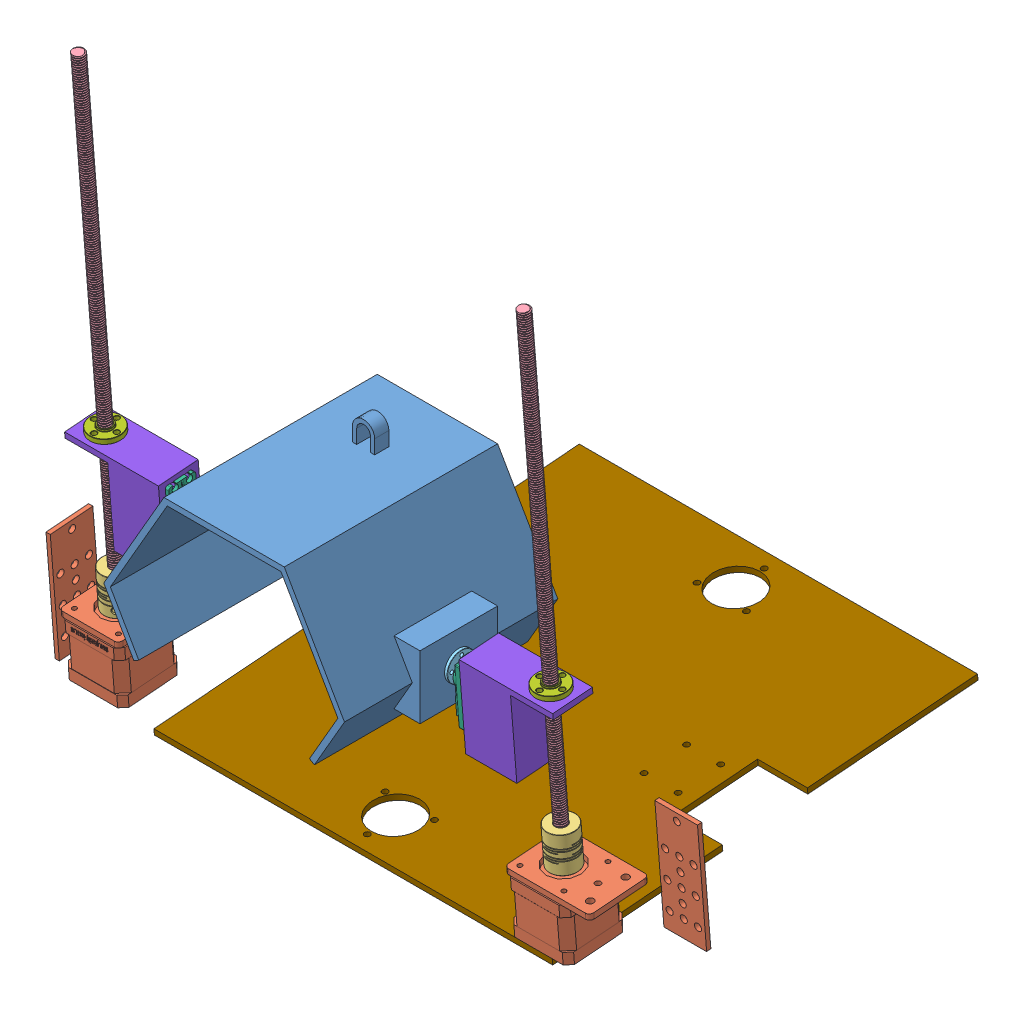
SolidWorks assembly robot, configuration Default. Lengths in mm.
Overall size (411.2 425.54 364.14).
16 component instances, 9 part files, 24 mates.
Components (placement in the parent):
- support element de jeu-1: support element de jeu [Default] at (45.2603 129.8077 131.4575) size (180 127.62 150)
- Holder nema17-1: Holder nema17 [По умолчанию] at (240.8603 32.8416 219.79) x (0 0.996834 0.079509) z (0 -0.079509 0.996834) size (89.57 60.3 80.06)
- NEMA17_Coupler-1: NEMA17_Coupler [Default] at (201.8603 38.4986 199.1745) x (-0.802928 0.047394 -0.594189) z (0.596077 0.06384 -0.800386) size (26.77 26 23.11)
- tige 8 mm-1: tige 8 mm [Varsayılan] at (201.8603 54.4479 200.4467) x (0.8944 -0.035562 0.445853) z (-0.447269 -0.071113 0.891568) size (8.04 340.5 9.24)
- MG955 horn-1: MG955 horn [Default] at (137.2603 129.8077 206.4575) x (0 1 0) z (0 0 1) size (20 4.5 20)
- ##Servo_MG_996R-1: ##Servo_MG_996R [Default] at (181.2603 119.8393 205.6624) x (0 0.996834 0.079509) z (0 -0.079509 0.996834) size (53.6 45.5 20)
- ecrou 8mm-1: ecrou 8mm [Default] at (201.8603 153.2333 208.326) x (-1 0 0) z (0 0.996834 0.079509) size (22 22 16.4)
- servo support-1: servo support [Default] at (150.8603 99.1075 214.0406) x (0 0.996834 0.079509) z (1 0 0) size (60 28 66)
- ##Servo_MG_996R-2: ##Servo_MG_996R [Default] at (-90.7397 119.8393 205.6624) x (0 0.996834 0.079509) z (0 0.079509 -0.996834) size (53.6 45.5 20)
- MG955 horn-2: MG955 horn [Default] at (-47.2397 129.8077 206.4575) x (0 1 0) z (0 0 1) size (20 4.5 20)
- servo support-2: servo support [Default] at (-60.3397 100.6977 194.1039) x (0 0.996834 0.079509) z (-1 0 0) size (60 28 66)
- ecrou 8mm-2: ecrou 8mm [Default] at (-111.3397 153.2333 208.326) x (-1 0 0) z (0 0.996834 0.079509) size (22 22 16.4)
- tige 8 mm-2: tige 8 mm [Varsayılan] at (-111.3049 54.4493 200.4293) x (0.8944 0.035562 -0.445853) z (0.447269 -0.071113 0.891568) size (8.04 340.5 9.24)
- NEMA17_Coupler-2: NEMA17_Coupler [Default] at (-111.3397 64.4163 201.2418) x (-0.802928 -0.047394 0.594189) z (0.596077 -0.06384 0.800386) size (26.77 26 23.11)
- Holder nema17-4: Holder nema17 [По умолчанию] at (-90.3397 37.6121 159.98) x (0 0.996834 0.079509) z (1 0 0) size (89.57 60.3 80.06)
- base-1: base [Default] at (71.1571 5.8914 67.164) x (-1 0 0) z (0 -0.996834 -0.079509) size (280 300 4)
Mates (geometry in assembly coordinates):
- Concentric1: concentric aligned: cylinder of Holder nema17-1 through (201.8603 58.4353 200.7647) axis (0 -0.996834 -0.079509) radius 2.495; cylinder of NEMA17_Coupler-1 through (201.8603 38.4986 199.1745) axis (0 -0.996834 -0.079509) radius 2.52
- Concentric2: concentric anti-aligned: cylinder of NEMA17_Coupler-1 through (201.8603 38.4986 199.1745) axis (0 -0.996834 -0.079509) radius 4.025; cylinder of 8mm trapez mil (1)-1 through (201.8603 54.4479 200.4467) axis (0 0.996834 0.079509) radius 3.1
- Coincident1: coincident anti-aligned: plane of support element de jeu-1 through (135.2603 129.8077 131.4575) normal (1 0 0); plane of MG955 horn-1 through (135.2603 129.8077 206.4575) normal (-1 0 0)
- Coincident3: coincident: point of support element de jeu-1; plane of MG955 horn-1 through (137.2603 129.8077 206.4575) normal (0 1 0)
- Concentric3: concentric anti-aligned: cylinder of MG955 horn-1 through (139.7603 129.8077 206.4575) axis (-1 0 0) radius 4.5; cylinder of ##Servo_MG_996R-1 through (135.7603 129.8077 206.4575) axis (1 0 0) radius 3
- Coincident4: coincident anti-aligned: plane of MG955 horn-1 through (139.7603 129.8077 206.4575) normal (1 0 0); plane of ##Servo_MG_996R-1 through (139.7603 129.8077 206.4575) normal (-1 0 0)
- Coincident10: coincident anti-aligned: plane of ##Servo_MG_996R-1 through (143.2603 140.5711 197.2843) normal (0 0.996834 0.079509); plane of servo support-1 through (182.8603 138.9809 217.2209) normal (0 -0.996834 -0.079509)
- Coincident11: coincident anti-aligned: plane of ##Servo_MG_996R-1 through (143.2603 99.1075 214.0406) normal (0 -0.079509 0.996834); plane of servo support-1 through (182.8603 99.1075 214.0406) normal (0 0.079509 -0.996834)
- Coincident12: coincident anti-aligned: plane of ##Servo_MG_996R-1 through (150.8603 119.8393 205.6624) normal (1 0 0); plane of servo support-1 through (150.8603 99.1075 214.0406) normal (-1 0 0)
- Concentric6: concentric aligned: cylinder of Trapezoidal lead screw Nut tr8x8-4 (1)-1 through (201.8603 139.776 207.2526) axis (0 0.996834 0.079509) radius 5.1; cylinder of servo support-1 through (201.8603 145.757 207.7297) axis (0 0.996834 0.079509) radius 5.5
- Coincident13: coincident anti-aligned: plane of Trapezoidal lead screw Nut tr8x8-4 (1)-1 through (201.8603 149.7443 208.0477) normal (0 -0.996834 -0.079509); plane of servo support-1 through (182.8603 148.6312 222.0034) normal (0 0.996834 0.079509)
- Parallel1: parallel anti-aligned: plane of Trapezoidal lead screw Nut tr8x8-4 (1)-1 through (201.8603 153.2333 208.326) normal (-1 0 0); plane of servo support-1 through (186.8603 99.1075 214.0406) normal (1 0 0)
- Concentric7: concentric aligned: cylinder of 8mm trapez mil (1)-1 through (201.8603 54.4479 200.4467) axis (0 0.996834 0.079509) radius 3.1; cylinder of Trapezoidal lead screw Nut tr8x8-4 (1)-1 through (201.8603 149.7443 208.0477) axis (0 0.996834 0.079509) radius 11
- Distance1: distance = 4 mm anti-aligned: plane of Holder nema17-1 through (201.8603 34.5113 198.8565) normal (0 0.996834 0.079509); plane of NEMA17_Coupler-1 through (199.6361 38.6299 197.5286) normal (0 -0.996834 -0.079509)
- Distance2: distance = 20 mm anti-aligned: plane of 8mm trapez mil (1)-1 through (201.8603 54.4479 200.4467) normal (0 -0.996834 -0.079509); plane of Holder nema17-1 through (201.8603 34.5113 198.8565) normal (0 0.996834 0.079509)
- Concentric8: concentric anti-aligned: cylinder of NEMA17_Coupler-2 through (-111.3397 64.4163 201.2418) axis (0 0.996834 0.079509) radius 4.025; cylinder of Holder nema17-4 through (-111.3397 58.4353 200.7647) axis (0 -0.996834 -0.079509) radius 2.495
- Coincident17: coincident aligned: plane of Holder nema17-1 through (240.8603 -6.035 216.6891) normal (0 -0.996834 -0.079509); plane of Holder nema17-4 through (-90.3397 -1.2644 156.8791) normal (0 -0.996834 -0.079509)
- Parallel2: parallel anti-aligned: plane of Holder nema17-1 through (181.0879 4.7973 181.4986) normal (-1 0 0); plane of Holder nema17-4 through (-90.2802 2.4349 211.1173) normal (1 0 0)
- Parallel3: parallel aligned: plane of Holder nema17-1 through (223.0879 2.412 211.4036) normal (1 0 0); plane of servo support-1 through (186.8603 99.1075 214.0406) normal (1 0 0)
- Coincident20: coincident: unknown of support element de jeu-1; plane of MG955 horn-1 through (137.2603 129.8077 206.4575) normal (0 1 0)
- Coincident22: coincident: unknown of support element de jeu-1; plane of MG955 horn-1 through (137.2603 129.8077 206.4575) normal (0 1 0)
- Coincident23: coincident: unknown of support element de jeu-1; plane of MG955 horn-1 through (137.2603 129.8077 206.4575) normal (0 0 1)
- Coincident24: coincident: plane of assembly; plane of Holder nema17-1 through (240.8603 -6.035 216.6891) normal (0 -0.996834 -0.079509); plane of base-1 through (71.1571 5.8914 67.164) normal (0 0.996834 0.079509)
- Coincident25: coincident: plane of Holder nema17-4 through (-128.3397 -6.035 216.6891) normal (0 -0.079509 0.996834); plane of base-1 through (221.1571 -10.0223 216.3711) normal (0 -0.079509 0.996834)
